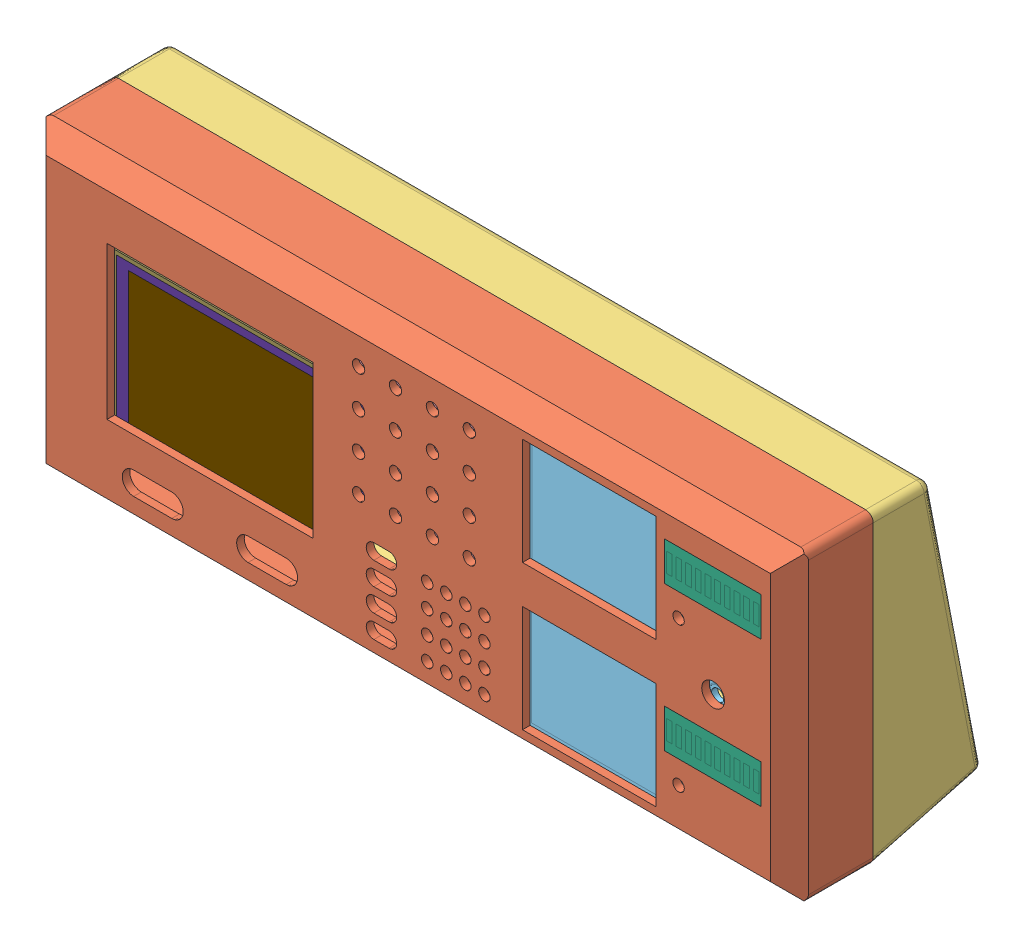
SolidWorks assembly Assem1, configuration Default. Lengths in mm.
Overall size (200 80 50.67).
49 component instances, 24 part files, 19 mates.
Components (placement in the parent):
- TFT LCD 2.4 inch ILI9341 touch-1: TFT LCD 2.4 inch ILI9341 touch [Default] at origin size (77.15 42.7 14.4)
  - TFT LCD 2.4 inch ILI9341 touch.step-1: TFT LCD 2.4 inch ILI9341 touch.step [Default] at origin size (77.15 42.7 14.4)
    - R1~R0603~R0603~HwOR.step-1: R1~R0603~R0603~HwOR.step [Default] at (51.3313 17.8702 0) x (0 -1 0) z (0 0 -1) size (1.62 0.81 0.45)
      - R0603~R0603~HwOR.step-1: R0603~R0603~HwOR.step [Default] at origin size (1.62 0.81 0.45)
    - C1~C0603~C0603_L1.6-W0.8-H0.8~HwOR.step-1: C1~C0603~C0603_L1.6-W0.8-H0.8~HwOR.step [Default] at (30.0394 8.9761 0) x (1 0 0) z (0 0 -1) size (1.6 0.8 0.8)
      - C0603~C0603_L1.6-W0.8-H0.8~HwOR.step-1: C0603~C0603_L1.6-W0.8-H0.8~HwOR.step [Default] at origin size (1.6 0.8 0.8)
    - H2~HDR-TH_4P-P2.54-V-M~HDR-TH_4P-P2.54-M-LI-1X4P~HwOR.step-1: H2~HDR-TH_4P-P2.54-V-M~HDR-TH_4P-P2.54-M-LI-1X4P~HwOR.step [Default] at (75.1801 25.1701 0) x (0 -1 0) z (0 0 -1) size (10.17 2.66 11.54)
      - HDR-TH_4P-P2.54-V-M~HDR-TH_4P-P2.54-M-LI-1X4P~HwOR.step-1: HDR-TH_4P-P2.54-V-M~HDR-TH_4P-P2.54-M-LI-1X4P~HwOR.step [Default] at origin size (10.17 2.66 11.54)
    - H3~CONN-TH_PZ254V-11-14P~CONN-TH_PZ254V-11-14P~HwOR.step-1: H3~CONN-TH_PZ254V-11-14P~CONN-TH_PZ254V-11-14P~HwOR.step [Default] at (2 4.85 0) x (0 1 0) z (0 0 -1) size (35.57 2.5 11.6)
      - CONN-TH_PZ254V-11-14P~CONN-TH_PZ254V-11-14P~HwOR.step-1: CONN-TH_PZ254V-11-14P~CONN-TH_PZ254V-11-14P~HwOR.step [Default] at origin size (35.57 2.5 11.6)
    - Q1~SOT-23-3_L2.9-W1.3-P1.90-LS2.4-BR~SOT-23-3P_L2.9-W1.3-H1.0-LS2.4-P0.95~HwOR.step-1: Q1~SOT-23-3_L2.9-W1.3-P1.90-LS2.4-BR~SOT-23-3P_L2.9-W1.3-H1.0-LS2.4-P0.95~HwOR.step [Default] at (19.5843 21.1653 0) x (-1 0 0) z (0 0 -1) size (2.5 2.89 1.06)
      - SOT-23-3_L2.9-W1.3-P1.90-LS2.4-BR~SOT-23-3P_L2.9-W1.3-H1.0-LS2.4-P0.95~HwOR.step-1: SOT-23-3_L2.9-W1.3-P1.90-LS2.4-BR~SOT-23-3P_L2.9-W1.3-H1.0-LS2.4-P0.95~HwOR.step [Default] at origin size (2.5 2.89 1.06)
    - U1~SD-CARD-SMD_SD-CARD-11P~SD-CARD-SMD_SD-CARD-11P~HwOR.step-1: U1~SD-CARD-SMD_SD-CARD-11P~SD-CARD-SMD_SD-CARD-11P~HwOR.step [Default] at (48.7311 32.7935 0) x (1 0 0) z (0 0 -1) size (27.7 17.71 3.85)
      - SD-CARD-SMD_SD-CARD-11P~SD-CARD-SMD_SD-CARD-11P~HwOR.step-1: SD-CARD-SMD_SD-CARD-11P~SD-CARD-SMD_SD-CARD-11P~HwOR.step [Default] at origin size (27.7 17.71 3.85)
    - U2~TSSOP-16_L5.0-W4.4-P0.65-LS6.4-BL~TSSOP-16_L5.0-W4.4-H1.0-LS6.4-P0.65~HwOR.step-1: U2~TSSOP-16_L5.0-W4.4-P0.65-LS6.4-BL~TSSOP-16_L5.0-W4.4-H1.0-LS6.4-P0.65~HwOR.step [Default] at (22.8993 6.6301 0) x (0 -1 0) z (0 0 -1) size (5 6.41 1.05)
      - TSSOP-16_L5.0-W4.4-P0.65-LS6.4-BL~TSSOP-16_L5.0-W4.4-H1.0-LS6.4-P0.65~HwOR.step-1: TSSOP-16_L5.0-W4.4-P0.65-LS6.4-BL~TSSOP-16_L5.0-W4.4-H1.0-LS6.4-P0.65~HwOR.step [Default] at origin size (5 6.41 1.05)
    - R1~R0603~R0603~HwOR.step-2: R1~R0603~R0603~HwOR.step [Default] at (48.6536 17.8702 0) x (0 -1 0) z (0 0 -1) size (1.62 0.81 0.45)
      - R0603~R0603~HwOR.step-1: R0603~R0603~HwOR.step [Default] at origin size (1.62 0.81 0.45)
    - R1~R0603~R0603~HwOR.step-3: R1~R0603~R0603~HwOR.step [Default] at (45.9973 17.8702 0) x (0 -1 0) z (0 0 -1) size (1.62 0.81 0.45)
      - R0603~R0603~HwOR.step-1: R0603~R0603~HwOR.step [Default] at origin size (1.62 0.81 0.45)
    - R1~R0603~R0603~HwOR.step-4: R1~R0603~R0603~HwOR.step [Default] at (16.535 21.1653 0) x (0 -1 0) z (0 0 -1) size (1.62 0.81 0.45)
      - R0603~R0603~HwOR.step-1: R0603~R0603~HwOR.step [Default] at origin size (1.62 0.81 0.45)
    - R1~R0603~R0603~HwOR.step-5: R1~R0603~R0603~HwOR.step [Default] at (16.6772 4.0801 0) x (0 -1 0) z (0 0 -1) size (1.62 0.81 0.45)
      - R0603~R0603~HwOR.step-1: R0603~R0603~HwOR.step [Default] at origin size (1.62 0.81 0.45)
    - R1~R0603~R0603~HwOR.step-6: R1~R0603~R0603~HwOR.step [Default] at (22.9395 21.1858 0) x (0 -1 0) z (0 0 -1) size (1.62 0.81 0.45)
      - R0603~R0603~HwOR.step-1: R0603~R0603~HwOR.step [Default] at origin size (1.62 0.81 0.45)
    - C1~C0603~C0603_L1.6-W0.8-H0.8~HwOR.step-2: C1~C0603~C0603_L1.6-W0.8-H0.8~HwOR.step [Default] at (22.7962 15.1258 0) x (0 -1 0) z (0 0 -1) size (1.6 0.8 0.8)
      - C0603~C0603_L1.6-W0.8-H0.8~HwOR.step-1: C0603~C0603_L1.6-W0.8-H0.8~HwOR.step [Default] at origin size (1.6 0.8 0.8)
    - Q1~SOT-23-3_L2.9-W1.3-P1.90-LS2.4-BR~SOT-23-3P_L2.9-W1.3-H1.0-LS2.4-P0.95~HwOR.step-2: Q1~SOT-23-3_L2.9-W1.3-P1.90-LS2.4-BR~SOT-23-3P_L2.9-W1.3-H1.0-LS2.4-P0.95~HwOR.step [Default] at (19.3803 15.2492 0) x (0 1 0) z (0 0 -1) size (2.5 2.89 1.06)
      - SOT-23-3_L2.9-W1.3-P1.90-LS2.4-BR~SOT-23-3P_L2.9-W1.3-H1.0-LS2.4-P0.95~HwOR.step-1: SOT-23-3_L2.9-W1.3-P1.90-LS2.4-BR~SOT-23-3P_L2.9-W1.3-H1.0-LS2.4-P0.95~HwOR.step [Default] at origin size (2.5 2.89 1.06)
    - Board~HwOR.step-1: Board~HwOR.step [Default] at origin size (77.15 42.69 1.6)
    - TopSilkscreen~HwOR.step-1: TopSilkscreen~HwOR.step [Default] at (0 0 1.6201) size (76.19 42.7 0.01)
    - BottomSilkscreen~HwOR.step-1: BottomSilkscreen~HwOR.step [Default] at (0 0 -0.02) size (75.96 41.18 0.02)
    - text.step-1: text.step [Default] at origin size (2.87 0.1 1)
    - EasyEDA PCB Model~HwOR.step-1: EasyEDA PCB Model~HwOR.step [Default] at origin size (60.51 42.69 4.2)
    - EasyEDA PCB Model~HwOR-0.step-1: EasyEDA PCB Model~HwOR-0.step [Default] at origin size (4.46 5.93 4.2)
    - EasyEDA PCB Model~HwOR-1.step-1: EasyEDA PCB Model~HwOR-1.step [Default] at origin size (4.45 0.59 4.2)
    - EasyEDA PCB Model~HwOR-2.step-1: EasyEDA PCB Model~HwOR-2.step [Default] at origin size (4.45 31.81 4.2)
    - EasyEDA PCB Model~HwOR-3.step-1: EasyEDA PCB Model~HwOR-3.step [Default] at origin size (4.45 0.62 4.2)
    - EasyEDA PCB Model~HwOR-4.step-1: EasyEDA PCB Model~HwOR-4.step [Default] at origin size (54.06 40.69 4.2)
    - EasyEDA PCB Model~HwOR-5.step-1: EasyEDA PCB Model~HwOR-5.step [Default] at origin size (48.96 36.72 4.2)
    - EasyEDA PCB Model~HwOR-6.step-1: EasyEDA PCB Model~HwOR-6.step [Default] at origin size (3.3 10.72 0.1)
- front-1: front [Default] at (0 0 6.3001) size (200 80 22)
- back-1: back [Default] at (-5.2562 0 6.3001) x (0 0 1) z (-1 0 0) size (28.66 80 200)
- Keypad-4x4-PB-1: Keypad-4x4-PB [Default] at (97.6675 35.0931 0.9001) x (0 1 0) z (1 0 0) size (43 8.5 39)
- 1.8 inch TFT Display SPI-1: 1.8 inch TFT Display SPI [Default] at (145.0576 41.1659 -3.0999) size (58 34.5 12.5)
- 1.8 inch TFT Display SPI-2: 1.8 inch TFT Display SPI [Default] at (145.0414 3.8382 -3.0999) size (58 34.5 12.5)
- LED Bar Graph Array-1: LED Bar Graph Array [Default] at (174.6438 46.5131 2.2201) x (0 1 0) z (0 0 1) size (10.17 26.17 9.09)
- LED Bar Graph Array-2: LED Bar Graph Array [Default] at (174.6438 8.5131 2.2201) x (0 1 0) z (0 0 1) size (10.17 26.17 9.09)
Mates (geometry in assembly coordinates):
- InPlace1: in place: plane of front-1 through (0 0 6.3001) normal (0 0 1); moOrthogonalPlaneRef_w of front-1 through (0 0 6.3001) normal (0 1 0); plane of front-1 through (0 0 6.3001) normal (1 0 0); unknown of front-1
- Coincident1: coincident aligned: 
- Coincident2: coincident aligned: plane of front-1 through (0 0 6.3001) normal (0 1 0)
- Coincident3: coincident anti-aligned: plane of front-1 through (0 0 6.3001) normal (1 0 0)
- InPlace2: in place: plane of front-1 through (-5.2562 -17.4069 -13.6999) normal (-1 0 0); plane of ? through (-5.2562 0 0) normal (-1 0 0); plane of front-1 through (-5.2562 -17.4069 -13.6999) normal (-1 0 0); plane of ? through (-5.2562 0 0) normal (0 1 0); plane of front-1 through (-5.2562 -17.4069 -13.6999) normal (-1 0 0); plane of ? through (-5.2562 0 0) normal (0 0 1); plane of front-1 through (-5.2562 -17.4069 -13.6999) normal (-1 0 0); unknown of back-1
- Coincident4: coincident aligned: plane of front-1; plane of back-1
- Coincident5: coincident aligned: moOrthogonalPlaneRef_w of front-1 through (-5.2562 0 6.3001) normal (0 1 0); plane of Part42^Assem1-1 through (-5.2562 0 6.3001) normal (0 1 0)
- Coincident6: coincident anti-aligned: moOrthogonalPlaneRef_w of front-1 through (-5.2562 0 6.3001) normal (0 0 -1); plane of Part42^Assem1-1 through (-5.2562 0 6.3001) normal (0 0 1)
- Distance1: distance = 1 mm anti-aligned: plane of Keypad-4x4-PB-1 through (84.7675 48.5781 5.3001) normal (0 0 1); plane of front-1 through (0 0 6.3001) normal (0 0 -1)
- Distance2: distance = 4 mm anti-aligned: plane of Keypad-4x4-PB-1 through (117.1675 56.5931 0.9001) normal (0 1 0); plane of front-1 through (194.7438 60.5931 -13.6999) normal (0 -1 0)
- Distance3: distance = 1 mm anti-aligned: plane of Keypad-4x4-PB-1 through (78.1675 56.5931 0.9001) normal (-1 0 0); plane of TFT LCD 2.4 inch ILI9341 touch-1/TFT LCD 2.4 inch ILI9341 touch.step-1/Board~HwOR.step-1 through (77.1675 42.7074 0) normal (1 0 0)
- Coincident2: coincident aligned: plane of TFT LCD 2.4 inch ILI9341 touch-1/TFT LCD 2.4 inch ILI9341 touch.step-1/EasyEDA PCB Model~HwOR-5.step-1 through (43.4275 21.3727 5.8001) normal (0 0 1); plane of 1.8 inch TFT Display SPI-1 through (142.9076 41.1659 5.8001) normal (0 0 1)
- Coincident3: coincident aligned: plane of 1.8 inch TFT Display SPI-1 through (142.9076 41.1659 5.8001) normal (0 0 1); plane of 1.8 inch TFT Display SPI-2 through (142.8914 3.8382 5.8001) normal (0 0 1)
- Coincident4: coincident aligned: plane of front-1 through (0 0 8.3001) normal (0 0 1); plane of LED Bar Graph Array-1 through (187.3438 41.4331 8.3001) normal (0 0 1)
- Coincident5: coincident aligned: plane of front-1 through (0 0 8.3001) normal (0 0 1); plane of LED Bar Graph Array-2 through (187.3438 3.4331 8.3001) normal (0 0 1)
- Coincident6: coincident anti-aligned: plane of front-1 through (161.9438 51.5931 6.3001) normal (0 -1 0); plane of LED Bar Graph Array-1 through (161.9438 51.5931 8.3001) normal (0 1 0)
- Coincident7: coincident anti-aligned: plane of front-1 through (161.9438 13.5931 6.3001) normal (0 -1 0); plane of LED Bar Graph Array-2 through (161.9438 13.5931 8.3001) normal (0 1 0)
- Coincident8: coincident anti-aligned: plane of front-1 through (161.9438 41.4331 6.3001) normal (1 0 0); plane of LED Bar Graph Array-1 through (161.9438 41.4331 8.3001) normal (-1 0 0)
- Coincident9: coincident anti-aligned: plane of front-1 through (161.9438 3.4331 6.3001) normal (1 0 0); plane of LED Bar Graph Array-2 through (161.9438 3.4331 8.3001) normal (-1 0 0)
